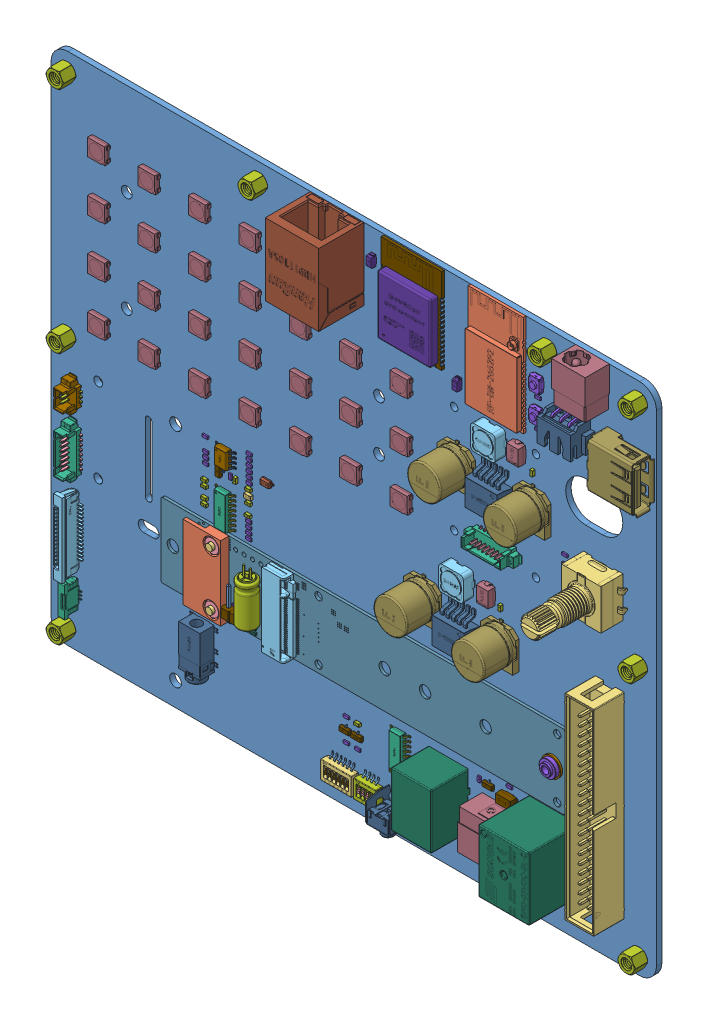
SolidWorks assembly HOUZZkitF1_Tester, configuration 默认. Lengths in mm. (continued)
Components (placement in the parent): (continued)
- HOUZZkitF1_Tester.step-1: HOUZZkitF1_Tester.step [默认] at origin size (180.06 153.05 26.45) (continued)
  - U5.step-1: U5.step [默认] at origin size (9.01 9.01 1.45) (continued)
    - LQFP48-7x7.step-1: LQFP48-7x7.step [默认] at (-10.2343 78.2414 -1.6) x (0 -1 0) z (0 0 -1) size (9.01 9.01 1.45) (continued)
      - ______0.25.step-27: ______0.25.step [默认] at (-3.5 -0.75 0.75) x (0 1 0) z (0 0 1) size (0.25 1 0.8)
      - ______0.25.step-28: ______0.25.step [默认] at (3.5 0.25 0.75) x (0 -1 0) z (0 0 1) size (0.25 1 0.8)
      - ______0.25.step-29: ______0.25.step [默认] at (-0.25 3.5 0.75) size (0.25 1 0.8)
      - ______0.25.step-30: ______0.25.step [默认] at (-3.5 -0.25 0.75) x (0 1 0) z (0 0 1) size (0.25 1 0.8)
      - ______0.25.step-31: ______0.25.step [默认] at (3.5 -0.25 0.75) x (0 -1 0) z (0 0 1) size (0.25 1 0.8)
      - ______0.25.step-32: ______0.25.step [默认] at (0.25 3.5 0.75) size (0.25 1 0.8)
      - ______0.25.step-33: ______0.25.step [默认] at (-3.5 0.25 0.75) x (0 1 0) z (0 0 1) size (0.25 1 0.8)
      - ______0.25.step-34: ______0.25.step [默认] at (3.5 -0.75 0.75) x (0 -1 0) z (0 0 1) size (0.25 1 0.8)
      - ______0.25.step-35: ______0.25.step [默认] at (0.75 3.5 0.75) size (0.25 1 0.8)
      - ______0.25.step-36: ______0.25.step [默认] at (-3.5 0.75 0.75) x (0 1 0) z (0 0 1) size (0.25 1 0.8)
      - ______0.25.step-37: ______0.25.step [默认] at (3.5 -1.25 0.75) x (0 -1 0) z (0 0 1) size (0.25 1 0.8)
      - ______0.25.step-38: ______0.25.step [默认] at (1.25 3.5 0.75) size (0.25 1 0.8)
      - ______0.25.step-39: ______0.25.step [默认] at (-3.5 1.25 0.75) x (0 1 0) z (0 0 1) size (0.25 1 0.8)
      - ______0.25.step-40: ______0.25.step [默认] at (3.5 -1.75 0.75) x (0 -1 0) z (0 0 1) size (0.25 1 0.8)
      - ______0.25.step-41: ______0.25.step [默认] at (1.75 3.5 0.75) size (0.25 1 0.8)
      - ______0.25.step-42: ______0.25.step [默认] at (-3.5 1.75 0.75) x (0 1 0) z (0 0 1) size (0.25 1 0.8)
      - ______0.25.step-43: ______0.25.step [默认] at (3.5 -2.25 0.75) x (0 -1 0) z (0 0 1) size (0.25 1 0.8)
      - ______0.25.step-44: ______0.25.step [默认] at (2.25 3.5 0.75) size (0.25 1 0.8)
      - ______0.25.step-45: ______0.25.step [默认] at (-3.5 2.25 0.75) x (0 1 0) z (0 0 1) size (0.25 1 0.8)
      - ______0.25.step-46: ______0.25.step [默认] at (3.5 -2.75 0.75) x (0 -1 0) z (0 0 1) size (0.25 1 0.8)
      - ______0.25.step-47: ______0.25.step [默认] at (2.75 3.5 0.75) size (0.25 1 0.8)
      - ______0.25.step-48: ______0.25.step [默认] at (-3.5 2.75 0.75) x (0 1 0) z (0 0 1) size (0.25 1 0.8)
      - LOGO__0.25-19.step-1: LOGO__0.25-19.step [默认] at origin size (0.75 0.87 0.01)
  - SW6.step-1: SW6.step [默认] at origin size (9.22 8.7 2.35)
    - CSW1.27-SMD-6P.step-1: CSW1.27-SMD-6P.step [默认] at (-3 -32 0) x (-1 0 0) z (0 0 1) size (9.22 8.7 2.35)
      - ______.step-1: ______.step [默认] at (3.175 0 1.55) x (-1 0 0) z (0 0 1) size (1 1.2 0.78)
      - ______-20.step-1: ______-20.step [默认] at (3.175 2.7 0.875) x (1 0 0) z (0 -1 0) size (0.4 0.95 1.65)
      - ______-20.step-2: ______-20.step [默认] at (3.175 -2.7 0.875) x (-1 0 0) z (0 1 0) size (0.4 0.95 1.65)
      - LOGO__0.25-21.step-1: LOGO__0.25-21.step [默认] at (0 0.0379 0.0475) x (1 0 0) z (0 0 -1) size (0.75 0.87 0.01)
      - ______-20.step-3: ______-20.step [默认] at (1.905 2.7 0.875) x (1 0 0) z (0 -1 0) size (0.4 0.95 1.65)
      - ______-20.step-4: ______-20.step [默认] at (0.635 2.7 0.875) x (1 0 0) z (0 -1 0) size (0.4 0.95 1.65)
      - ______-20.step-5: ______-20.step [默认] at (1.905 -2.7 0.875) x (-1 0 0) z (0 1 0) size (0.4 0.95 1.65)
      - ______-20.step-6: ______-20.step [默认] at (0.635 -2.7 0.875) x (-1 0 0) z (0 1 0) size (0.4 0.95 1.65)
      - ______.step-2: ______.step [默认] at (1.905 0 1.55) x (-1 0 0) z (0 0 1) size (1 1.2 0.78)
      - ______.step-3: ______.step [默认] at (0.635 0 1.55) x (-1 0 0) z (0 0 1) size (1 1.2 0.78)
      - ______-20.step-7: ______-20.step [默认] at (-0.635 2.7 0.875) x (1 0 0) z (0 -1 0) size (0.4 0.95 1.65)
      - ______.step-4: ______.step [默认] at (-0.635 0 1.55) x (-1 0 0) z (0 0 1) size (1 1.2 0.78)
      - ______-20.step-8: ______-20.step [默认] at (-0.635 -2.7 0.875) x (-1 0 0) z (0 1 0) size (0.4 0.95 1.65)
      - ______.step-5: ______.step [默认] at (-1.905 0 1.55) x (-1 0 0) z (0 0 1) size (1 1.2 0.78)
      - ______-20.step-9: ______-20.step [默认] at (-1.905 2.7 0.875) x (1 0 0) z (0 -1 0) size (0.4 0.95 1.65)
      - ______-20.step-10: ______-20.step [默认] at (-1.905 -2.7 0.875) x (-1 0 0) z (0 1 0) size (0.4 0.95 1.65)
      - CSW1.27-SMD-6P-22.step-1: CSW1.27-SMD-6P-22.step [默认] at origin size (9.22 5.4 2.3)
      - ______-20.step-11: ______-20.step [默认] at (-3.175 2.7 0.875) x (1 0 0) z (0 -1 0) size (0.4 0.95 1.65)
      - ______.step-6: ______.step [默认] at (-3.175 0 1.55) x (-1 0 0) z (0 0 1) size (1 1.2 0.78)
      - ______-20.step-12: ______-20.step [默认] at (-3.175 -2.7 0.875) x (-1 0 0) z (0 1 0) size (0.4 0.95 1.65)
  - SW5.step-1: SW5.step [默认] at origin size (6.68 8.7 2.35)
    - CSW1.27-SMD-4P.step-1: CSW1.27-SMD-4P.step [默认] at (5.5 -32 0) x (-1 0 0) z (0 0 1) size (6.68 8.7 2.35)
      - ______-23.step-1: ______-23.step [默认] at (1.9 0 1.55) x (-1 0 0) z (0 0 1) size (1 1.2 0.78)
      - ______-24.step-1: ______-24.step [默认] at (1.905 2.7 0.875) x (1 0 0) z (0 -1 0) size (0.4 0.95 1.65)
      - ______-24.step-2: ______-24.step [默认] at (1.905 -2.7 0.875) x (-1 0 0) z (0 1 0) size (0.4 0.95 1.65)
      - LOGO__0.25-25.step-1: LOGO__0.25-25.step [默认] at (0 0.0379 0.0475) x (1 0 0) z (0 0 -1) size (0.75 0.87 0.01)
      - ______-24.step-3: ______-24.step [默认] at (0.635 2.7 0.875) x (1 0 0) z (0 -1 0) size (0.4 0.95 1.65)
      - ______-24.step-4: ______-24.step [默认] at (-0.635 2.7 0.875) x (1 0 0) z (0 -1 0) size (0.4 0.95 1.65)
      - ______-24.step-5: ______-24.step [默认] at (0.635 -2.7 0.875) x (-1 0 0) z (0 1 0) size (0.4 0.95 1.65)
      - ______-24.step-6: ______-24.step [默认] at (-0.635 -2.7 0.875) x (-1 0 0) z (0 1 0) size (0.4 0.95 1.65)
      - ______-23.step-2: ______-23.step [默认] at (0.63 0 1.55) x (-1 0 0) z (0 0 1) size (1 1.2 0.78)
      - ______-23.step-3: ______-23.step [默认] at (-0.64 0 1.55) x (-1 0 0) z (0 0 1) size (1 1.2 0.78)
      - CSW1.27-SMD-4P-26.step-1: CSW1.27-SMD-4P-26.step [默认] at origin size (6.68 5.4 2.3)
      - ______-24.step-7: ______-24.step [默认] at (-1.905 2.7 0.875) x (1 0 0) z (0 -1 0) size (0.4 0.95 1.65)
      - ______-23.step-4: ______-23.step [默认] at (-1.91 0 1.55) x (-1 0 0) z (0 0 1) size (1 1.2 0.78)
      - ______-24.step-8: ______-24.step [默认] at (-1.905 -2.7 0.875) x (-1 0 0) z (0 1 0) size (0.4 0.95 1.65)
  - SW4.step-1: SW4.step [默认] at origin size (3 4.4 2)
    - SW3x4.step-1: SW3x4.step [默认] at (62.9504 92.6578 -1.6) x (0 -1 0) z (0 0 1) size (4.4 3 2)
      - 3D_PCB1_2022-09-07.step.step-1: 3D_PCB1_2022-09-07.step.step [默认] at origin size (4.4 3 2)
        - SW1.step.step-1: SW1.step.step [默认] at (2.9502 -7.9502 1.6001) size (4.4 3 2)
          - SW-SMD_ST-1185U.step.step-1: SW-SMD_ST-1185U.step.step [默认] at origin size (4.4 3 2)
            - COMPOUND.step.step-1: COMPOUND.step.step [默认] at origin size (4.4 3 2)
  - SW3.step-1: SW3.step [默认] at origin size (3 4.4 2)
    - SW3x4.step-1: SW3x4.step [默认] at (47.0496 94.9422 -1.6) x (0 1 0) z (0 0 1) size (4.4 3 2)
      - 3D_PCB1_2022-09-07.step.step-1: 3D_PCB1_2022-09-07.step.step [默认] at origin size (4.4 3 2)
        - SW1.step.step-1: SW1.step.step [默认] at (2.9502 -7.9502 1.6001) size (4.4 3 2)
          - SW-SMD_ST-1185U.step.step-1: SW-SMD_ST-1185U.step.step [默认] at origin size (4.4 3 2)
            - COMPOUND.step.step-1: COMPOUND.step.step [默认] at origin size (4.4 3 2)
  - SW2.step-1: SW2.step [默认] at origin size (8.37 8.85 10.88)
    - TSW DIP-6x6x6_V.step-1: TSW DIP-6x6x6_V.step [默认] at (14.25 -31.873 0.1) x (1 0 0) z (0 -1 0) size (8.37 10.88 8.85)
      - LOGO__-27.step-1: LOGO__-27.step [默认] at (-0.0217 0.921 0.5803) x (1 0 0) z (0 -1 0) size (1.2 1.38 0.01)
      - TSW DIP-6x6x6_V-28.step-1: TSW DIP-6x6x6_V-28.step [默认] at origin size (8.37 10.88 8.85)
  - RJ1.step-1: RJ1.step [默认] at origin size (15.88 21.4 16.5)
    - HanRun-HR911105A.step-1: HanRun-HR911105A.step [默认] at (2.9712 112.9265 13.4) x (-1 0 0) z (0 1 0) size (15.88 16.5 21.4)
  - R28.step-1: R28.step [默认] at origin size (1.6 0.8 0.4)
    - R 0603.step-1: R 0603.step [默认] at (46.5001 -10.4999 0) x (1 0 0) z (0 0 1) size (1.6 0.8 0.4)
      - R 0603-5.step-1: R 0603-5.step [默认] at origin size (1.6 0.8 0.4)
      - LOGO__-6.step-1: LOGO__-6.step [默认] at (0.0001 0.0322 -0.0016) x (-1 0 0) z (0 0 -1) size (0.48 0.55 0)
  - R27.step-1: R27.step [默认] at origin size (0.8 1.6 0.4)
    - R 0603.step-1: R 0603.step [默认] at (37.5 -12.9999 0) x (0 1 0) z (0 0 1) size (1.6 0.8 0.4)
      - R 0603-5.step-1: R 0603-5.step [默认] at origin size (1.6 0.8 0.4)
      - LOGO__-6.step-1: LOGO__-6.step [默认] at (0.0001 0.0322 -0.0016) x (-1 0 0) z (0 0 -1) size (0.48 0.55 0)
  - R26.step-1: R26.step [默认] at origin size (0.8 1.6 0.4)
    - R 0603.step-1: R 0603.step [默认] at (-15.4 87.7001 -1.6) x (0 1 0) z (0 0 -1) size (1.6 0.8 0.4)
      - R 0603-5.step-1: R 0603-5.step [默认] at origin size (1.6 0.8 0.4)
      - LOGO__-6.step-1: LOGO__-6.step [默认] at (0.0001 0.0322 -0.0016) x (-1 0 0) z (0 0 -1) size (0.48 0.55 0)
  - R25.step-1: R25.step [默认] at origin size (0.8 1.6 0.4)
    - R 0603.step-1: R 0603.step [默认] at (-18.6001 87.6999 -1.6) x (0 -1 0) z (0 0 -1) size (1.6 0.8 0.4)
      - R 0603-5.step-1: R 0603-5.step [默认] at origin size (1.6 0.8 0.4)
      - LOGO__-6.step-1: LOGO__-6.step [默认] at (0.0001 0.0322 -0.0016) x (-1 0 0) z (0 0 -1) size (0.48 0.55 0)
  - R24.step-1: R24.step [默认] at origin size (0.8 1.6 0.4)
    - R 0603.step-1: R 0603.step [默认] at (-9.8001 87.6999 -1.6) x (0 -1 0) z (0 0 -1) size (1.6 0.8 0.4)
      - R 0603-5.step-1: R 0603-5.step [默认] at origin size (1.6 0.8 0.4)
      - LOGO__-6.step-1: LOGO__-6.step [默认] at (0.0001 0.0322 -0.0016) x (-1 0 0) z (0 0 -1) size (0.48 0.55 0)
  - R23.step-1: R23.step [默认] at origin size (0.8 1.6 0.4)
    - R 0603.step-1: R 0603.step [默认] at (-8.2001 87.6999 -1.6) x (0 -1 0) z (0 0 -1) size (1.6 0.8 0.4)
      - R 0603-5.step-1: R 0603-5.step [默认] at origin size (1.6 0.8 0.4)
      - LOGO__-6.step-1: LOGO__-6.step [默认] at (0.0001 0.0322 -0.0016) x (-1 0 0) z (0 0 -1) size (0.48 0.55 0)
  - R22.step-1: R22.step [默认] at origin size (0.8 1.6 0.4)
    - R 0603.step-1: R 0603.step [默认] at (-17.0001 87.6999 -1.6) x (0 -1 0) z (0 0 -1) size (1.6 0.8 0.4)
      - R 0603-5.step-1: R 0603-5.step [默认] at origin size (1.6 0.8 0.4)
      - LOGO__-6.step-1: LOGO__-6.step [默认] at (0.0001 0.0322 -0.0016) x (-1 0 0) z (0 0 -1) size (0.48 0.55 0)
  - R21.step-1: R21.step [默认] at origin size (0.8 1.6 0.4)
    - R 0603.step-1: R 0603.step [默认] at (-3.4001 87.6999 -1.6) x (0 -1 0) z (0 0 -1) size (1.6 0.8 0.4)
      - R 0603-5.step-1: R 0603-5.step [默认] at origin size (1.6 0.8 0.4)
      - LOGO__-6.step-1: LOGO__-6.step [默认] at (0.0001 0.0322 -0.0016) x (-1 0 0) z (0 0 -1) size (0.48 0.55 0)
  - R20.step-1: R20.step [默认] at origin size (0.8 1.6 0.4)
    - R 0603.step-1: R 0603.step [默认] at (-0.2001 87.6999 -1.6) x (0 -1 0) z (0 0 -1) size (1.6 0.8 0.4)
      - R 0603-5.step-1: R 0603-5.step [默认] at origin size (1.6 0.8 0.4)
      - LOGO__-6.step-1: LOGO__-6.step [默认] at (0.0001 0.0322 -0.0016) x (-1 0 0) z (0 0 -1) size (0.48 0.55 0)
  - R19.step-1: R19.step [默认] at origin size (0.8 1.6 0.4)
    - R 0603.step-1: R 0603.step [默认] at (1.3999 87.6999 -1.6) x (0 -1 0) z (0 0 -1) size (1.6 0.8 0.4)
      - R 0603-5.step-1: R 0603-5.step [默认] at origin size (1.6 0.8 0.4)
      - LOGO__-6.step-1: LOGO__-6.step [默认] at (0.0001 0.0322 -0.0016) x (-1 0 0) z (0 0 -1) size (0.48 0.55 0)
  - R18.step-1: R18.step [默认] at origin size (0.8 1.6 0.4)
    - R 0603.step-1: R 0603.step [默认] at (-6.4866 69.9684 -1.6) x (0 1 0) z (0 0 -1) size (1.6 0.8 0.4)
      - R 0603-5.step-1: R 0603-5.step [默认] at origin size (1.6 0.8 0.4)
      - LOGO__-6.step-1: LOGO__-6.step [默认] at (0.0001 0.0322 -0.0016) x (-1 0 0) z (0 0 -1) size (0.48 0.55 0)
  - R17.step-1: R17.step [默认] at origin size (1.6 0.8 0.4)
    - R 0603.step-1: R 0603.step [默认] at (-18.8197 83.4196 -1.6) x (-1 0 0) z (0 0 -1) size (1.6 0.8 0.4)
      - R 0603-5.step-1: R 0603-5.step [默认] at origin size (1.6 0.8 0.4)
      - LOGO__-6.step-1: LOGO__-6.step [默认] at (0.0001 0.0322 -0.0016) x (-1 0 0) z (0 0 -1) size (0.48 0.55 0)
  - R16.step-1: R16.step [默认] at origin size (1.6 0.8 0.4)
    - R 0603.step-1: R 0603.step [默认] at (-18.8197 81.864 -1.6) x (-1 0 0) z (0 0 -1) size (1.6 0.8 0.4)
      - R 0603-5.step-1: R 0603-5.step [默认] at origin size (1.6 0.8 0.4)
      - LOGO__-6.step-1: LOGO__-6.step [默认] at (0.0001 0.0322 -0.0016) x (-1 0 0) z (0 0 -1) size (0.48 0.55 0)
  - R15.step-1: R15.step [默认] at origin size (1.6 0.8 0.4)
    - R 0603.step-1: R 0603.step [默认] at (-18.8197 80.3084 -1.6) x (-1 0 0) z (0 0 -1) size (1.6 0.8 0.4)
      - R 0603-5.step-1: R 0603-5.step [默认] at origin size (1.6 0.8 0.4)
      - LOGO__-6.step-1: LOGO__-6.step [默认] at (0.0001 0.0322 -0.0016) x (-1 0 0) z (0 0 -1) size (0.48 0.55 0)
  - R14.step-1: R14.step [默认] at origin size (0.8 1.6 0.4)
    - R 0603.step-1: R 0603.step [默认] at (-13.3456 70.0389 -1.6) x (0 -1 0) z (0 0 -1) size (1.6 0.8 0.4)
      - R 0603-5.step-1: R 0603-5.step [默认] at origin size (1.6 0.8 0.4)
      - LOGO__-6.step-1: LOGO__-6.step [默认] at (0.0001 0.0322 -0.0016) x (-1 0 0) z (0 0 -1) size (0.48 0.55 0)
  - R13.step-1: R13.step [默认] at origin size (0.8 1.6 0.4)
    - R 0603.step-1: R 0603.step [默认] at (-21.7188 75.8535 -1.6) x (0 -1 0) z (0 0 -1) size (1.6 0.8 0.4)
      - R 0603-5.step-1: R 0603-5.step [默认] at origin size (1.6 0.8 0.4)
      - LOGO__-6.step-1: LOGO__-6.step [默认] at (0.0001 0.0322 -0.0016) x (-1 0 0) z (0 0 -1) size (0.48 0.55 0)
  - R12.step-1: R12.step [默认] at origin size (1.6 0.8 0.4)
    - R 0603.step-1: R 0603.step [默认] at (63.0002 52.5001 0) x (1 0 0) z (0 0 1) size (1.6 0.8 0.4)
      - R 0603-5.step-1: R 0603-5.step [默认] at origin size (1.6 0.8 0.4)
      - LOGO__-6.step-1: LOGO__-6.step [默认] at (0.0001 0.0322 -0.0016) x (-1 0 0) z (0 0 -1) size (0.48 0.55 0)
  - R10.step-1: R10.step [默认] at origin size (1.6 0.8 0.4)
    - R 0603.step-1: R 0603.step [默认] at (63.0001 55.0001 0) x (1 0 0) z (0 0 1) size (1.6 0.8 0.4)
      - R 0603-5.step-1: R 0603-5.step [默认] at origin size (1.6 0.8 0.4)
      - LOGO__-6.step-1: LOGO__-6.step [默认] at (0.0001 0.0322 -0.0016) x (-1 0 0) z (0 0 -1) size (0.48 0.55 0)
  - R9.step-1: R9.step [默认] at origin size (1.6 0.8 0.4)
    - R 0603.step-1: R 0603.step [默认] at (55.0001 85.7001 0) x (1 0 0) z (0 0 1) size (1.6 0.8 0.4)
      - R 0603-5.step-1: R 0603-5.step [默认] at origin size (1.6 0.8 0.4)
      - LOGO__-6.step-1: LOGO__-6.step [默认] at (0.0001 0.0322 -0.0016) x (-1 0 0) z (0 0 -1) size (0.48 0.55 0)
  - R8.step-1: R8.step [默认] at origin size (1.6 0.8 0.4)
    - R 0603.step-1: R 0603.step [默认] at (55.0001 94.0001 0) x (1 0 0) z (0 0 1) size (1.6 0.8 0.4)
      - R 0603-5.step-1: R 0603-5.step [默认] at origin size (1.6 0.8 0.4)
      - LOGO__-6.step-1: LOGO__-6.step [默认] at (0.0001 0.0322 -0.0016) x (-1 0 0) z (0 0 -1) size (0.48 0.55 0)
  - R7.step-1: R7.step [默认] at origin size (1.6 0.8 0.4)
    - R 0603.step-1: R 0603.step [默认] at (-1.9999 -23.3999 0) x (1 0 0) z (0 0 1) size (1.6 0.8 0.4)
      - R 0603-5.step-1: R 0603-5.step [默认] at origin size (1.6 0.8 0.4)
      - LOGO__-6.step-1: LOGO__-6.step [默认] at (0.0001 0.0322 -0.0016) x (-1 0 0) z (0 0 -1) size (0.48 0.55 0)
  - R6.step-1: R6.step [默认] at origin size (1.6 0.8 0.4)
    - R 0603.step-1: R 0603.step [默认] at (1.3999 -23.4 0) x (-1 0 0) z (0 0 1) size (1.6 0.8 0.4)
      - R 0603-5.step-1: R 0603-5.step [默认] at origin size (1.6 0.8 0.4)
      - LOGO__-6.step-1: LOGO__-6.step [默认] at (0.0001 0.0322 -0.0016) x (-1 0 0) z (0 0 -1) size (0.48 0.55 0)
  - R5.step-1: R5.step [默认] at origin size (1.6 0.8 0.4)
    - R 0603.step-1: R 0603.step [默认] at (-1.9999 -16.6999 0) size (1.6 0.8 0.4)
      - R 0603-5.step-1: R 0603-5.step [默认] at origin size (1.6 0.8 0.4)
      - LOGO__-6.step-1: LOGO__-6.step [默认] at (0.0001 0.0322 -0.0016) x (-1 0 0) z (0 0 -1) size (0.48 0.55 0)
  - Q3.step-1: Q3.step [默认] at origin size (3 2.4 1.05)
    - SOT23-3.step-1: SOT23-3.step [默认] at (40.5 -13 0) x (1 0 0) z (0 0 1) size (3 2.4 1.05)
      - SOT23-3-10.step-1: SOT23-3-10.step [默认] at origin size (3 1.3 1)
      - SOT23-3 ______.step-1: SOT23-3 ______.step [默认] at (0 0.5461 0.475) size (0.4 0.65 0.55)
      - SOT23-3 ______.step-2: SOT23-3 ______.step [默认] at (-0.95 -0.5461 0.475) x (-1 0 0) z (0 0 1) size (0.4 0.65 0.55)
      - SOT23-3 ______.step-3: SOT23-3 ______.step [默认] at (0.95 -0.5461 0.475) x (-1 0 0) z (0 0 1) size (0.4 0.65 0.55)
      - LOGO__0.15.step-1: LOGO__0.15.step [默认] at (0 -0.0163 0.0485) x (-1 0 0) z (0 0 -1) size (0.45 0.52 0)
  - Q2.step-1: Q2.step [默认] at origin size (3 2.4 1.05)
    - SOT23-3.step-1: SOT23-3.step [默认] at (1.5 -20 0) x (1 0 0) z (0 0 1) size (3 2.4 1.05)
      - SOT23-3-10.step-1: SOT23-3-10.step [默认] at origin size (3 1.3 1)
      - SOT23-3 ______.step-1: SOT23-3 ______.step [默认] at (0 0.5461 0.475) size (0.4 0.65 0.55)
      - SOT23-3 ______.step-2: SOT23-3 ______.step [默认] at (-0.95 -0.5461 0.475) x (-1 0 0) z (0 0 1) size (0.4 0.65 0.55)
      - SOT23-3 ______.step-3: SOT23-3 ______.step [默认] at (0.95 -0.5461 0.475) x (-1 0 0) z (0 0 1) size (0.4 0.65 0.55)
      - LOGO__0.15.step-1: LOGO__0.15.step [默认] at (0 -0.0163 0.0485) x (-1 0 0) z (0 0 -1) size (0.45 0.52 0)
  - Q1.step-1: Q1.step [默认] at origin size (3 2.4 1.05)
    - SOT23-3.step-1: SOT23-3.step [默认] at (-2 -20 0) x (1 0 0) z (0 0 1) size (3 2.4 1.05)
      - SOT23-3-10.step-1: SOT23-3-10.step [默认] at origin size (3 1.3 1)
      - SOT23-3 ______.step-1: SOT23-3 ______.step [默认] at (0 0.5461 0.475) size (0.4 0.65 0.55)
      - SOT23-3 ______.step-2: SOT23-3 ______.step [默认] at (-0.95 -0.5461 0.475) x (-1 0 0) z (0 0 1) size (0.4 0.65 0.55)
      - SOT23-3 ______.step-3: SOT23-3 ______.step [默认] at (0.95 -0.5461 0.475) x (-1 0 0) z (0 0 1) size (0.4 0.65 0.55)
      - LOGO__0.15.step-1: LOGO__0.15.step [默认] at (0 -0.0163 0.0485) x (-1 0 0) z (0 0 -1) size (0.45 0.52 0)
  - LED26.step-1: LED26.step [默认] at origin size (0.8 1.6 0.61)
    - LED 0603-B.step-1: LED 0603-B.step [默认] at (-14.972 70.1096 -1.6) x (0 1 0) z (0 0 -1) size (1.6 0.8 0.47)
      - LED 0603-B-29.step-1: LED 0603-B-29.step [默认] at origin size (1.6 0.8 0.47)
      - LOGO__-30.step-1: LOGO__-30.step [默认] at (0 0.0303 -0.002) x (-1 0 0) z (0 0 -1) size (0.6 0.69 0)
    - LED 0603____g___RGB16711680.step-1: LED 0603____g___RGB16711680.step [默认] at (-14.9721 70.1097 -1.6) x (0 -1 0) z (0 0 -1) size (1.2 0.8 0.4)
  - LB1.step-1: LB1.step [默认] at origin size (1.21 2.01 0.91)
    - FB 0805.step-1: FB 0805.step [默认] at (-8.3958 70.039 -1.6) x (0 1 0) z (-1 0 0) size (2 0.91 1.2)
      - FB 0805-11.step-1: FB 0805-11.step [默认] at origin size (2 0.91 1.2)
      - LOGO__0.15-12.step-1: LOGO__0.15-12.step [默认] at (-0.0107 -0.0015 -0.0162) x (1 0 0) z (0 1 0) size (0.45 0.52 0)
  - JK1.step-1: JK1.step [默认] at origin size (15.09 18.69 18.66)
    - SRD-03VDC-SL-C.step-1: SRD-03VDC-SL-C.step [默认] at (59.5001 -19.4001 0) x (0 1 0) z (0 0 1) size (18.69 15.09 18.66)
  - IC1.step-1: IC1.step [默认] at origin size (6.01 10 1.9)
    - SOP16.step-1: SOP16.step [默认] at (14 -17 0) x (-1 0 0) z (0 0 1) size (6.01 10 1.9)
      - LOGO__0.25.step-1: LOGO__0.25.step [默认] at (0.0116 0 0.095) x (0 -1 0) z (0 0 -1) size (0.75 0.87 0.01)
      - SOP16 ____.step-1: SOP16 ____.step [默认] at origin size (3.6 10 1.8)
      - ________1.8 ____________.step-1: ________1.8 ____________.step [默认] at (1.8 4.45 1) x (0 1 0) z (0 0 1) size (0.5 1.2 1.1)
      - ________1.8 ____________.step-2: ________1.8 ____________.step [默认] at (1.8 3.18 1) x (0 1 0) z (0 0 1) size (0.5 1.2 1.1)
      - ________1.8 ____________.step-3: ________1.8 ____________.step [默认] at (1.8 1.91 1) x (0 1 0) z (0 0 1) size (0.5 1.2 1.1)
      - ________1.8 ____________.step-4: ________1.8 ____________.step [默认] at (1.8 0.64 1) x (0 1 0) z (0 0 1) size (0.5 1.2 1.1)
      - ________1.8 ____________.step-5: ________1.8 ____________.step [默认] at (1.8 -0.63 1) x (0 1 0) z (0 0 1) size (0.5 1.2 1.1)
      - ________1.8 ____________.step-6: ________1.8 ____________.step [默认] at (1.8 -1.9 1) x (0 1 0) z (0 0 1) size (0.5 1.2 1.1)
      - ________1.8 ____________.step-7: ________1.8 ____________.step [默认] at (1.8 -3.17 1) x (0 1 0) z (0 0 1) size (0.5 1.2 1.1)
      - ________1.8 ____________.step-8: ________1.8 ____________.step [默认] at (1.8 -4.44 1) x (0 1 0) z (0 0 1) size (0.5 1.2 1.1)
      - ________1.8 ____________.step-9: ________1.8 ____________.step [默认] at (-1.8 4.45 1) x (0 -1 0) z (0 0 1) size (0.5 1.2 1.1)
      - ________1.8 ____________.step-10: ________1.8 ____________.step [默认] at (-1.8 3.18 1) x (0 -1 0) z (0 0 1) size (0.5 1.2 1.1)
      - ________1.8 ____________.step-11: ________1.8 ____________.step [默认] at (-1.8 1.91 1) x (0 -1 0) z (0 0 1) size (0.5 1.2 1.1)
      - ________1.8 ____________.step-12: ________1.8 ____________.step [默认] at (-1.8 0.64 1) x (0 -1 0) z (0 0 1) size (0.5 1.2 1.1)
      - ________1.8 ____________.step-13: ________1.8 ____________.step [默认] at (-1.8 -0.63 1) x (0 -1 0) z (0 0 1) size (0.5 1.2 1.1)
      - ________1.8 ____________.step-14: ________1.8 ____________.step [默认] at (-1.8 -1.9 1) x (0 -1 0) z (0 0 1) size (0.5 1.2 1.1)
      - ________1.8 ____________.step-15: ________1.8 ____________.step [默认] at (-1.8 -3.17 1) x (0 -1 0) z (0 0 1) size (0.5 1.2 1.1)
      - ________1.8 ____________.step-16: ________1.8 ____________.step [默认] at (-1.8 -4.44 1) x (0 -1 0) z (0 0 1) size (0.5 1.2 1.1)
  - E3.step-1: E3.step [默认] at origin size (1.6 3.2 1.61)
    - CD A(3216).step-1: CD A(3216).step [默认] at (31.5 86 0) x (0 -1 0) z (0 0 1) size (3.2 1.6 1.61)
      - LOGO__-31.step-1: LOGO__-31.step [默认] at (0 0.0355 -0.005) x (-1 0 0) z (0 0 -1) size (0.75 0.87 0.01)
      - CD A(3216)-32.step-1: CD A(3216)-32.step [默认] at (0 0 0.8) size (3.2 1.6 1.6)
  - E2.step-1: E2.step [默认] at origin size (1.6 3.2 1.61)
    - CD A(3216).step-1: CD A(3216).step [默认] at (6 105 0) x (0 1 0) z (0 0 1) size (3.2 1.6 1.61)
      - LOGO__-31.step-1: LOGO__-31.step [默认] at (0 0.0355 -0.005) x (-1 0 0) z (0 0 -1) size (0.75 0.87 0.01)
      - CD A(3216)-32.step-1: CD A(3216)-32.step [默认] at (0 0 0.8) size (3.2 1.6 1.6)
  - D1.step-1: D1.step [默认] at origin size (5.12 2.6 2.11)
    - SMA.step-1: SMA.step [默认] at (46.5229 -13.4999 0.05) x (-1 0 0) z (0 0 1) size (5.12 2.6 2.11)
      - SMA-33.step-1: SMA-33.step [默认] at origin size (5.12 2.6 2.1)
      - LOGO__________.____-34.step-1: LOGO__________.____-34.step [默认] at (0.0018 0.0048 -0.003) x (-1 0 0) z (0 0 -1) size (0.9 1.04 0.01)
  - CF2.step-1: CF2.step [默认] at origin size (0.82 1.6 0.82)
    - C 0603.step-1: C 0603.step [默认] at (53.5 74 0) x (0 -1 0) z (0 0 1) size (1.6 0.82 0.82)
      - LOGO__-3.step-1: LOGO__-3.step [默认] at (0 0.0171 -0.0006) x (-1 0 0) z (0 0 -1) size (0.51 0.59 0)
      - C 0603-4.step-1: C 0603-4.step [默认] at origin size (1.6 0.82 0.82)
  - CF1.step-1: CF1.step [默认] at origin size (0.82 1.6 0.82)
    - C 0603.step-1: C 0603.step [默认] at (44 34.5 0) x (0 -1 0) z (0 0 1) size (1.6 0.82 0.82)
      - LOGO__-3.step-1: LOGO__-3.step [默认] at (0 0.0171 -0.0006) x (-1 0 0) z (0 0 -1) size (0.51 0.59 0)
      - C 0603-4.step-1: C 0603-4.step [默认] at origin size (1.6 0.82 0.82)
  - C17.step-1: C17.step [默认] at origin size (1.62 3.2 1.22)
    - C 1206.step-1: C 1206.step [默认] at (-13.4 87.7 -1.6) x (0 1 0) z (0 0 -1) size (3.2 1.62 1.22)
      - LOGO__-35.step-1: LOGO__-35.step [默认] at (0 0.0171 -0.0006) x (-1 0 0) z (0 0 -1) size (0.51 0.59 0)
      - C 1206-36.step-1: C 1206-36.step [默认] at origin size (3.2 1.62 1.22)
  - C16.step-1: C16.step [默认] at origin size (0.82 1.6 0.82)
    - C 0603.step-1: C 0603.step [默认] at (-6.6 87.7 -1.6) x (0 1 0) z (0 0 -1) size (1.6 0.82 0.82)
      - LOGO__-3.step-1: LOGO__-3.step [默认] at (0 0.0171 -0.0006) x (-1 0 0) z (0 0 -1) size (0.51 0.59 0)
      - C 0603-4.step-1: C 0603-4.step [默认] at origin size (1.6 0.82 0.82)
  - C15.step-1: C15.step [默认] at origin size (0.82 1.6 0.82)
    - C 0603.step-1: C 0603.step [默认] at (-5 87.7 -1.6) x (0 1 0) z (0 0 -1) size (1.6 0.82 0.82)
      - LOGO__-3.step-1: LOGO__-3.step [默认] at (0 0.0171 -0.0006) x (-1 0 0) z (0 0 -1) size (0.51 0.59 0)
      - C 0603-4.step-1: C 0603-4.step [默认] at origin size (1.6 0.82 0.82)
  - C14.step-1: C14.step [默认] at origin size (0.82 1.6 0.82)
    - C 0603.step-1: C 0603.step [默认] at (-11.4 87.7 -1.6) x (0 -1 0) z (0 0 -1) size (1.6 0.82 0.82)
      - LOGO__-3.step-1: LOGO__-3.step [默认] at (0 0.0171 -0.0006) x (-1 0 0) z (0 0 -1) size (0.51 0.59 0)
      - C 0603-4.step-1: C 0603-4.step [默认] at origin size (1.6 0.82 0.82)
  - C13.step-1: C13.step [默认] at origin size (0.82 1.6 0.82)
    - C 0603.step-1: C 0603.step [默认] at (-1.8 87.7 -1.6) x (0 -1 0) z (0 0 -1) size (1.6 0.82 0.82)
      - LOGO__-3.step-1: LOGO__-3.step [默认] at (0 0.0171 -0.0006) x (-1 0 0) z (0 0 -1) size (0.51 0.59 0)
      - C 0603-4.step-1: C 0603-4.step [默认] at origin size (1.6 0.82 0.82)
  - C12.step-1: C12.step [默认] at origin size (0.82 1.6 0.82)
    - C 0603.step-1: C 0603.step [默认] at (-18.1539 70.039 -1.6) x (0 -1 0) z (0 0 -1) size (1.6 0.82 0.82)
      - LOGO__-3.step-1: LOGO__-3.step [默认] at (0 0.0171 -0.0006) x (-1 0 0) z (0 0 -1) size (0.51 0.59 0)
      - C 0603-4.step-1: C 0603-4.step [默认] at origin size (1.6 0.82 0.82)
  - C11.step-1: C11.step [默认] at origin size (0.82 1.6 0.82)
    - C 0603.step-1: C 0603.step [默认] at (-16.5983 70.039 -1.6) x (0 -1 0) z (0 0 -1) size (1.6 0.82 0.82)
      - LOGO__-3.step-1: LOGO__-3.step [默认] at (0 0.0171 -0.0006) x (-1 0 0) z (0 0 -1) size (0.51 0.59 0)
      - C 0603-4.step-1: C 0603-4.step [默认] at origin size (1.6 0.82 0.82)
  - C10.step-1: C10.step [默认] at origin size (0.82 1.6 0.82)
    - C 0603.step-1: C 0603.step [默认] at (-11.79 70.039 -1.6) x (0 1 0) z (0 0 -1) size (1.6 0.82 0.82)
      - LOGO__-3.step-1: LOGO__-3.step [默认] at (0 0.0171 -0.0006) x (-1 0 0) z (0 0 -1) size (0.51 0.59 0)
      - C 0603-4.step-1: C 0603-4.step [默认] at origin size (1.6 0.82 0.82)
  - C9.step-1: C9.step [默认] at origin size (0.82 1.6 0.82)
    - C 0603.step-1: C 0603.step [默认] at (-10.2343 70.039 -1.6) x (0 1 0) z (0 0 -1) size (1.6 0.82 0.82)
      - LOGO__-3.step-1: LOGO__-3.step [默认] at (0 0.0171 -0.0006) x (-1 0 0) z (0 0 -1) size (0.51 0.59 0)
      - C 0603-4.step-1: C 0603-4.step [默认] at origin size (1.6 0.82 0.82)
  - C8.step-1: C8.step [默认] at origin size (1.6 0.82 0.82)
    - C 0603.step-1: C 0603.step [默认] at (-18.8196 78.7527 -1.6) x (1 0 0) z (0 0 -1) size (1.6 0.82 0.82)
      - LOGO__-3.step-1: LOGO__-3.step [默认] at (0 0.0171 -0.0006) x (-1 0 0) z (0 0 -1) size (0.51 0.59 0)
      - C 0603-4.step-1: C 0603-4.step [默认] at origin size (1.6 0.82 0.82)
  - C7.step-1: C7.step [默认] at origin size (1.6 0.82 0.82)
    - C 0603.step-1: C 0603.step [默认] at (-18.8196 72.6716 -1.6) x (-1 0 0) z (0 0 -1) size (1.6 0.82 0.82)
      - LOGO__-3.step-1: LOGO__-3.step [默认] at (0 0.0171 -0.0006) x (-1 0 0) z (0 0 -1) size (0.51 0.59 0)
      - C 0603-4.step-1: C 0603-4.step [默认] at origin size (1.6 0.82 0.82)
  - C6.step-1: C6.step [默认] at origin size (1.6 0.82 0.82)
    - C 0603.step-1: C 0603.step [默认] at (12 -23.5 0) x (-1 0 0) z (0 0 1) size (1.6 0.82 0.82)
      - LOGO__-3.step-1: LOGO__-3.step [默认] at (0 0.0171 -0.0006) x (-1 0 0) z (0 0 -1) size (0.51 0.59 0)
      - C 0603-4.step-1: C 0603-4.step [默认] at origin size (1.6 0.82 0.82)
  - C5.step-1: C5.step [默认] at origin size (1.6 0.82 0.82)
    - C 0603.step-1: C 0603.step [默认] at (1.5 -16.7 0) x (-1 0 0) z (0 0 1) size (1.6 0.82 0.82)
      - LOGO__-3.step-1: LOGO__-3.step [默认] at (0 0.0171 -0.0006) x (-1 0 0) z (0 0 -1) size (0.51 0.59 0)
      - C 0603-4.step-1: C 0603-4.step [默认] at origin size (1.6 0.82 0.82)
  - JP7.step-1: JP7.step [默认] at origin size (15.15 4.1 4.7)
    - MOLEX1.25-LS-8P.step-1: MOLEX1.25-LS-8P.step [默认] at (42.5 50 0) x (-1 0 0) z (0 0 1) size (15.15 4.1 4.7)
      - MOLEX1.25-LS-______.step-1: MOLEX1.25-LS-______.step [默认] at (4.375 0.45 0.75) x (0 -1 0) z (0 0 1) size (3.7 0.32 3.85)
      - MOLEX1.25-LS-______.step-2: MOLEX1.25-LS-______.step [默认] at (3.125 0.45 0.75) x (0 -1 0) z (0 0 1) size (3.7 0.32 3.85)
      - MOLEX1.25-LS-______.step-3: MOLEX1.25-LS-______.step [默认] at (1.875 0.45 0.75) x (0 -1 0) z (0 0 1) size (3.7 0.32 3.85)
      - MOLEX1.25-LS-______.step-4: MOLEX1.25-LS-______.step [默认] at (0.625 0.45 0.75) x (0 -1 0) z (0 0 1) size (3.7 0.32 3.85)
      - MOLEX1.25-LS-______.step-5: MOLEX1.25-LS-______.step [默认] at (-0.625 0.45 0.75) x (0 -1 0) z (0 0 1) size (3.7 0.32 3.85)
      - MOLEX1.25-LS-______.step-6: MOLEX1.25-LS-______.step [默认] at (-1.875 0.45 0.75) x (0 -1 0) z (0 0 1) size (3.7 0.32 3.85)
      - MOLEX1.25-LS-______.step-7: MOLEX1.25-LS-______.step [默认] at (-3.125 0.45 0.75) x (0 -1 0) z (0 0 1) size (3.7 0.32 3.85)
      - MOLEX1.25-LS-______.step-8: MOLEX1.25-LS-______.step [默认] at (-4.375 0.45 0.75) x (0 -1 0) z (0 0 1) size (3.7 0.32 3.85)
      - LOGO__0.15-37.step-1: LOGO__0.15-37.step [默认] at (5.035 0.4556 0.247) size (0.45 0.52 0)
      - MOLEX1.25-LS-8P-38.step-1: MOLEX1.25-LS-8P-38.step [默认] at origin size (15.15 3.6 4.7)
  - SP10.step-1: SP10.step [默认] at origin size (5.4 5.23 4.07)
    - M3x4.step-1: M3x4.step [默认] at (85 40 0) x (1 0 0) z (0 0 1) size (5.4 5.23 4.07)
  - SP9.step-1: SP9.step [默认] at origin size (5.4 5.23 4.07)
    - M3x4.step-1: M3x4.step [默认] at (-85 40 0) x (1 0 0) z (0 0 1) size (5.4 5.23 4.07)
  - SP6.step-1: SP6.step [默认] at origin size (5.4 5.23 4.07)
    - M3x4.step-1: M3x4.step [默认] at (58 108 0) x (1 0 0) z (0 0 1) size (5.4 5.23 4.07)
  - SP5.step-1: SP5.step [默认] at origin size (5.4 5.23 4.07)
    - M3x4.step-1: M3x4.step [默认] at (-28 108 0) x (1 0 0) z (0 0 1) size (5.4 5.23 4.07)
  - JP6.step-1: JP6.step [默认] at origin size (12.5 10.42 6.06)
    - XH2.54-WS-3P.step-1: XH2.54-WS-3P.step [默认] at (65.5 92 0) size (12.5 10.42 6.06)
      - XH2.54-WS-______.step-1: XH2.54-WS-______.step [默认] at (-2.5 3.35 3.85) x (-1 0 0) z (0 0 1) size (0.7 9.07 4.21)
      - XH2.54-WS-______.step-2: XH2.54-WS-______.step [默认] at (0 3.35 3.85) x (-1 0 0) z (0 0 1) size (0.7 9.07 4.21)
      - LOGO__0.5-39.step-1: LOGO__0.5-39.step [默认] at (-0.027 -0.0593 0.24) size (1.5 1.73 0.01)
      - XH2.54-WS-3P-40.step-1: XH2.54-WS-3P-40.step [默认] at origin size (12.5 8 6.05)
      - XH2.54-WS-______.step-3: XH2.54-WS-______.step [默认] at (2.5 3.35 3.85) x (-1 0 0) z (0 0 1) size (0.7 9.07 4.21)
  - SP4.step-1: SP4.step [默认] at origin size (5.4 5.23 4.07)
    - M3x4.step-1: M3x4.step [默认] at (85 -35 0) x (1 0 0) z (0 0 1) size (5.4 5.23 4.07)
  - SP3.step-1: SP3.step [默认] at origin size (5.4 5.23 4.07)
    - M3x4.step-1: M3x4.step [默认] at (-85 -35 0) x (1 0 0) z (0 0 1) size (5.4 5.23 4.07)
  - SP2.step-1: SP2.step [默认] at origin size (5.4 5.23 4.07)
    - M3x4.step-1: M3x4.step [默认] at (85 108 0) x (1 0 0) z (0 0 1) size (5.4 5.23 4.07)
  - SP1.step-1: SP1.step [默认] at origin size (5.4 5.23 4.07)
    - M3x4.step-1: M3x4.step [默认] at (-85 108 0) x (1 0 0) z (0 0 1) size (5.4 5.23 4.07)
  - H4.step-1: H4.step [默认] at origin size (25.31 29.5 2.85)
    - tfcard_test_wire_female.step-1: tfcard_test_wire_female.step [默认] at (-76 20 -1.6) x (0 -1 0) z (0 0 -1) size (29.5 25.31 2.85)
      - MICRO SD CARD SOCKET.step-1: MICRO SD CARD SOCKET.step [默认] at (119.8236 -42.8675 -195.6897) size (16 17.9 2.44)
        - MICRO SD CARD SOCKET.step.step-1: MICRO SD CARD SOCKET.step.step [默认] at origin size (16 17.9 2.44)
          - micro sd.step.step-1: micro sd.step.step [默认] at origin size (16 17.9 2.44)
            - micro sd_1.step.step-1: micro sd_1.step.step [默认] at origin size (16 17.9 2.44)
              - sd (1).step.step-1: sd (1).step.step [默认] at origin size (11 15 1.1)
                - sd.step.step-1: sd.step.step [默认] at (-74.7886 45.5089 197.5397) x (-1 0 0) z (0 0 1) size (11 15 1.1)
              - slot (1).step.step-1: slot (1).step.step [默认] at origin size (16 15 2.44)
                - slot.step.step-1: slot.step.step [默认] at (-120.4736 47.0914 197.5397) x (-1 0 0) z (0 0 1) size (16 15 2.44)
          - MOV_SD.step.step-1: MOV_SD.step.step [默认] at origin size (0.7 0.5 0.1)
          - MOV_SD-0.step.step-1: MOV_SD-0.step.step [默认] at origin size (0.7 0.5 0.1)
          - MOV_SD-1.step.step-1: MOV_SD-1.step.step [默认] at origin size (0.7 0.5 0.1)
          - MOV_SD-2.step.step-1: MOV_SD-2.step.step [默认] at origin size (0.7 0.5 0.1)
          - MOV_SD-3.step.step-1: MOV_SD-3.step.step [默认] at origin size (0.7 0.5 0.1)
          - MOV_SD-4.step.step-1: MOV_SD-4.step.step [默认] at origin size (0.7 0.5 0.1)
          - MOV_SD-5.step.step-1: MOV_SD-5.step.step [默认] at origin size (0.7 0.5 0.1)
          - MOV_SD-6.step.step-1: MOV_SD-6.step.step [默认] at origin size (0.7 0.5 0.1)
          - MOV_SD-7.step.step-1: MOV_SD-7.step.step [默认] at origin size (0.7 0.5 0.1)
          - MOV_SD-8.step.step-1: MOV_SD-8.step.step [默认] at origin size (0.97 0.18 0.1)
          - MOV_SD-9.step.step-1: MOV_SD-9.step.step [默认] at origin size (1.3 1.04 0.1)
          - MOV_SD-10.step.step-1: MOV_SD-10.step.step [默认] at origin size (0.97 0.89 0.1)
          - MOV_SD-11.step.step-1: MOV_SD-11.step.step [默认] at origin size (0.97 0.91 0.1)
          - MOV_SD-12.step.step-1: MOV_SD-12.step.step [默认] at origin size (0.97 0.52 0.1)
